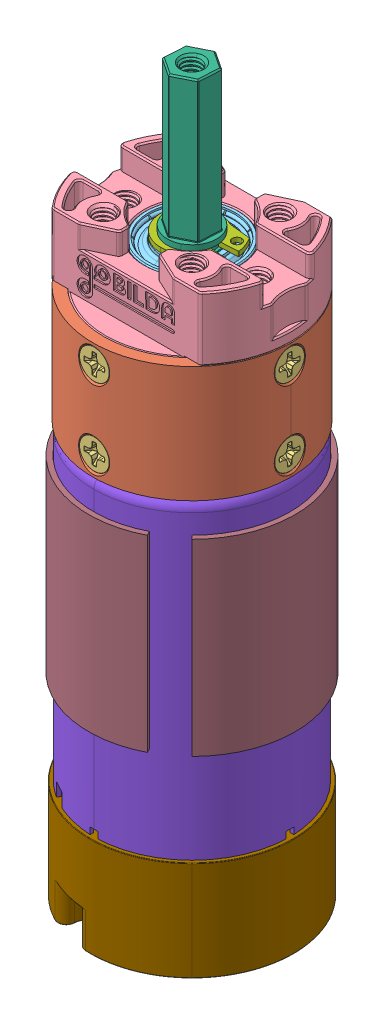
SolidWorks assembly 电机, configuration 默认. Lengths in mm.
Overall size (52.29 131.17 52.29).
30 component instances, 15 part files, 0 mates.
Components (placement in the parent):
- 5203-2402-0001 assembly.STEP-1: 5203-2402-0001 assembly.STEP [默认] at origin size (52.29 131.17 52.29)
  - 5103-2402-0001 Simple.STEP-1: 5103-2402-0001 Simple.STEP [默认] at (21.5499 39.1 -25.8711) size (36 56.22 35.96)
    - 5103 Gearbox Base.STEP-1: 5103 Gearbox Base.STEP [默认] at (-58.7206 21.0354 14.7927) size (31.9 5.6 31.9)
    - 5103 Gearbox Barrel (1 stage, simple)_Gear Blank.STEP-1: 5103 Gearbox Barrel (1 stage, simple)_Gear Blank.STEP [默认] at (-58.7206 55.1554 14.7927) x (1 0 0) z (0 -1 0) size (35.96 35.96 21.12)
    - 5103 Gearbox Barrel Screw (M3 x 8mm length Flat Head)_92010A118.STEP-1: 5103 Gearbox Barrel Screw (M3 x 8mm length Flat Head)_92010A118.STEP [默认] at (-58.7206 24.5354 30.8757) x (0.002439 -0.999997 0) z (0 0 1) size (5.46 5.46 8.04)
    - 5103 Gearbox Barrel Screw (M3 x 8mm length Flat Head)_92010A118.STEP-2: 5103 Gearbox Barrel Screw (M3 x 8mm length Flat Head)_92010A118.STEP [默认] at (-58.7206 38.6554 30.8757) x (-0.002439 -0.999997 0) z (0 0 1) size (5.46 5.46 8.04)
    - 5103 Gearbox Barrel Screw (M3 x 8mm length Flat Head)_92010A118.STEP-3: 5103 Gearbox Barrel Screw (M3 x 8mm length Flat Head)_92010A118.STEP [默认] at (-42.6376 24.5354 14.7927) x (0 -0.999997 -0.002439) z (1 0 0) size (5.46 5.46 8.04)
    - 5103 Gearbox Barrel Screw (M3 x 8mm length Flat Head)_92010A118.STEP-4: 5103 Gearbox Barrel Screw (M3 x 8mm length Flat Head)_92010A118.STEP [默认] at (-58.7206 24.5354 -1.2903) x (-0.002439 -0.999997 0) z (0 0 -1) size (5.46 5.46 8.04)
    - 5103 Gearbox Barrel Screw (M3 x 8mm length Flat Head)_92010A118.STEP-5: 5103 Gearbox Barrel Screw (M3 x 8mm length Flat Head)_92010A118.STEP [默认] at (-74.8037 24.5354 14.7927) x (0 -0.999997 0.002439) z (-1 0 0) size (5.46 5.46 8.04)
    - 5103 Gearbox Barrel Screw (M3 x 8mm length Flat Head)_92010A118.STEP-6: 5103 Gearbox Barrel Screw (M3 x 8mm length Flat Head)_92010A118.STEP [默认] at (-42.6376 38.6554 14.7927) x (0 -0.999997 0.002439) z (1 0 0) size (5.46 5.46 8.04)
    - 5103 Gearbox Barrel Screw (M3 x 8mm length Flat Head)_92010A118.STEP-7: 5103 Gearbox Barrel Screw (M3 x 8mm length Flat Head)_92010A118.STEP [默认] at (-58.7206 38.6554 -1.2903) x (0.002439 -0.999997 0) z (0 0 -1) size (5.46 5.46 8.04)
    - 5103 Gearbox Barrel Screw (M3 x 8mm length Flat Head)_92010A118.STEP-8: 5103 Gearbox Barrel Screw (M3 x 8mm length Flat Head)_92010A118.STEP [默认] at (-74.8037 38.6554 14.7927) x (0 -0.999997 -0.002439) z (-1 0 0) size (5.46 5.46 8.04)
    - 5103 Gearbox Face.STEP-1: 5103 Gearbox Face.STEP [默认] at (-58.7206 36.6554 14.7927) size (36 17.1 31.9)
    - 5103 Gearbox Bearing.STEP-1: 5103 Gearbox Bearing.STEP [默认] at (-58.7206 44.7554 14.7927) size (17 5 17)
    - 5103 Gearbox Bearing.STEP-2: 5103 Gearbox Bearing.STEP [默认] at (-58.7206 36.6554 14.7927) size (17 5 17)
    - 5103 Gearbox Shaft (23.5mm Length, Simple).STEP-1: 5103 Gearbox Shaft (23.5mm Length, Simple).STEP [默认] at (-58.7206 33.2954 14.7927) x (0.894773 0 -0.44652) z (0.44652 0 0.894773) size (8.97 40.6 8.97)
    - 5103 Gearbox Snap Ring.STEP-1: 5103 Gearbox Snap Ring.STEP [默认] at (-58.7206 49.8304 14.7927) x (0 1 0) z (0 0 1) size (0.85 13.06 10.66)
  - 5000-0002-0001 body.STEP-1: 5000-0002-0001 body.STEP [默认] at (-37.1707 3.4854 -11.0784) size (35.61 61.45 35.61)
  - 5000-0001-0001 encoder cap.STEP-1: 5000-0001-0001 encoder cap.STEP [默认] at (-37.1707 -14.6146 -11.0784) x (0.707107 0 -0.707107) z (0 -1 0) size (36.9 36.9 18.3)
  - 5000-0001-0001 encoder cap screw_90190A075.STEP-1: 5000-0001-0001 encoder cap screw_90190A075.STEP [默认] at (-33.0775 -8.1646 -26.1474) x (0.882398 0 0.470504) z (0 -1 0) size (3.33 3.33 7.86)
  - 5000-0001-0001 encoder pin housing.STEP-1: 5000-0001-0001 encoder pin housing.STEP [默认] at (-44.0085 -0.9746 -21.9467) x (0.707107 0 -0.707107) z (-0.707107 0 -0.707107) size (12.3 7.19 6.3)
  - 5000-0001-0001 encoder pins_MalePinHeader_1X2.STEP-1: 5000-0001-0001 encoder pins_MalePinHeader_1X2.STEP [默认] at (-43.4569 1.2544 -23.1912) x (0.707107 0 -0.707107) z (0 -1 0) size (3.18 0.64 4.27)
  - 5000-0001-0001 motor shield.STEP-1: 5000-0001-0001 motor shield.STEP [默认] at (-37.1707 54.6354 -11.0784) x (0.808104 0 -0.58904) z (0 -1 0) size (37.5 37.27 34.15)
  - 5000-0001-0001 encoder cap screw_90190A075.STEP-2: 5000-0001-0001 encoder cap screw_90190A075.STEP [默认] at (-41.264 -8.1646 3.9905) x (0.882398 0 0.470504) z (0 -1 0) size (3.33 3.33 7.86)
  - 5000-0001-0001 encoder pins_MalePinHeader_1X2.STEP-2: 5000-0001-0001 encoder pins_MalePinHeader_1X2.STEP [默认] at (-47.049 1.2544 -19.5991) x (0.707107 0 -0.707107) z (0 -1 0) size (3.18 0.64 4.27)
  - 5000-0002-0117 motor shaft.STEP-1: 5000-0002-0117 motor shaft.STEP [默认] at (-37.1707 59.4854 -11.0784) size (3.26 12.53 3.14)
  - 5103 Gearbox Base Mounting Screw M3 x 5mm length SHCS)_91290A110.STEP-1: 5103 Gearbox Base Mounting Screw M3 x 5mm length SHCS)_91290A110.STEP [默认] at (-46.0096 57.2554 -2.2396) x (0.056382 0 0.998409) z (0 -1 0) size (5.5 5.5 8.14)
  - 5103 Gearbox Base Mounting Screw M3 x 5mm length SHCS)_91290A110.STEP-2: 5103 Gearbox Base Mounting Screw M3 x 5mm length SHCS)_91290A110.STEP [默认] at (-28.3319 57.2554 -2.2396) x (0.998409 0 -0.056382) z (0 -1 0) size (5.5 5.5 8.14)
  - 5103 Gearbox Base Mounting Screw M3 x 5mm length SHCS)_91290A110.STEP-3: 5103 Gearbox Base Mounting Screw M3 x 5mm length SHCS)_91290A110.STEP [默认] at (-28.3319 57.2554 -19.9173) x (-0.056382 0 -0.998409) z (0 -1 0) size (5.5 5.5 8.14)
  - 5103 Gearbox Base Mounting Screw M3 x 5mm length SHCS)_91290A110.STEP-4: 5103 Gearbox Base Mounting Screw M3 x 5mm length SHCS)_91290A110.STEP [默认] at (-46.0096 57.2554 -19.9173) x (-0.998409 0 0.056382) z (0 -1 0) size (5.5 5.5 8.14)
